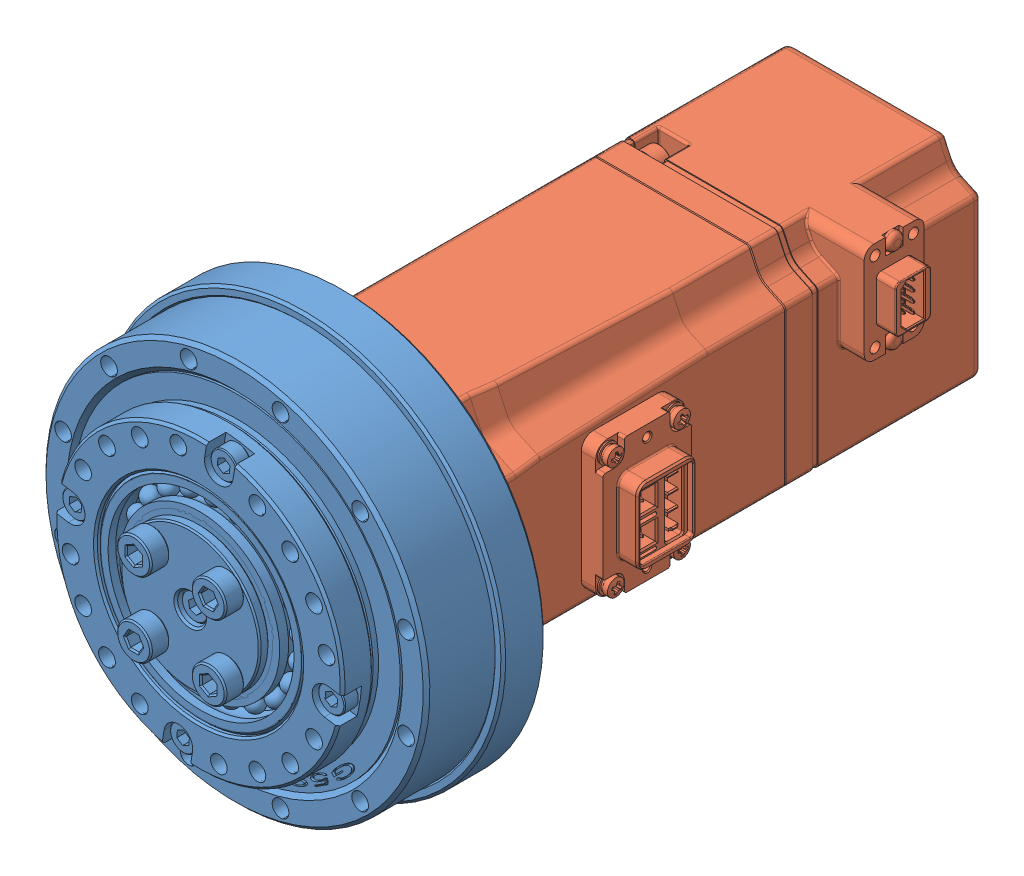
SolidWorks assembly Servo_100W_ZXF17, configuration По умолчанию. Lengths in mm.
Overall size (84 84 149.26).
2 component instances, 2 part files, 7 mates.
Components (placement in the parent):
- ZXF17_40-1: ZXF17_40 [По умолчанию] at (0 0 -30.5)
- Серва 100W FL 40 ELM1H-0100MA40E 95.3-1: Серва 100W FL 40 ELM1H-0100MA40E 95.3 [По умолчанию] at (0 0 17.2301) x (0 -1 0) z (0 0 1)
Mates (geometry in assembly coordinates):
- Совпадение1: coincident aligned: plane of ZXF17_40-1 through (0 0 0) normal (0 0 1)
- Совпадение2: coincident aligned: plane of ZXF17_40-1 through (0 0 -30.5) normal (0 1 0)
- Совпадение3: coincident aligned: plane of ZXF17_40-1 through (0 0 -30.5) normal (1 0 0)
- Концентричный1: concentric aligned: cylinder of ZXF17_40-1 through (0 0 -30) axis (0 0 1) radius 15; cylinder of Серва 100W FL 40 ELM1H-0100MA40E 95.3-1 through (0 0 -20.1425) axis (0 0 1) radius 15
- Концентричный2: concentric aligned: line of ZXF17_40-1 through (16.2635 16.2635 -30.5) axis (0 0 -1); cylinder of Серва 100W FL 40 ELM1H-0100MA40E 95.3-1 through (16.2635 16.2635 -27.499) axis (0 0 -1) radius 2.25
- Совпадение4: coincident anti-aligned: plane of ZXF17_40-1 through (0 0 -30.5) normal (0 0 -1); plane of Серва 100W FL 40 ELM1H-0100MA40E 95.3-1 through (-15 0 -30.5) normal (0 0 1)
- Совпадение9: coincident anti-aligned: plane of Серва 100W FL 40 ELM1H-0100MA40E 95.3-1 through (-15.5 0 -35.5) normal (0 0 -1); plane of Шайба DIN 127_v2-1 through (13.7789 19.1387 -35.5) normal (0 0 1)
